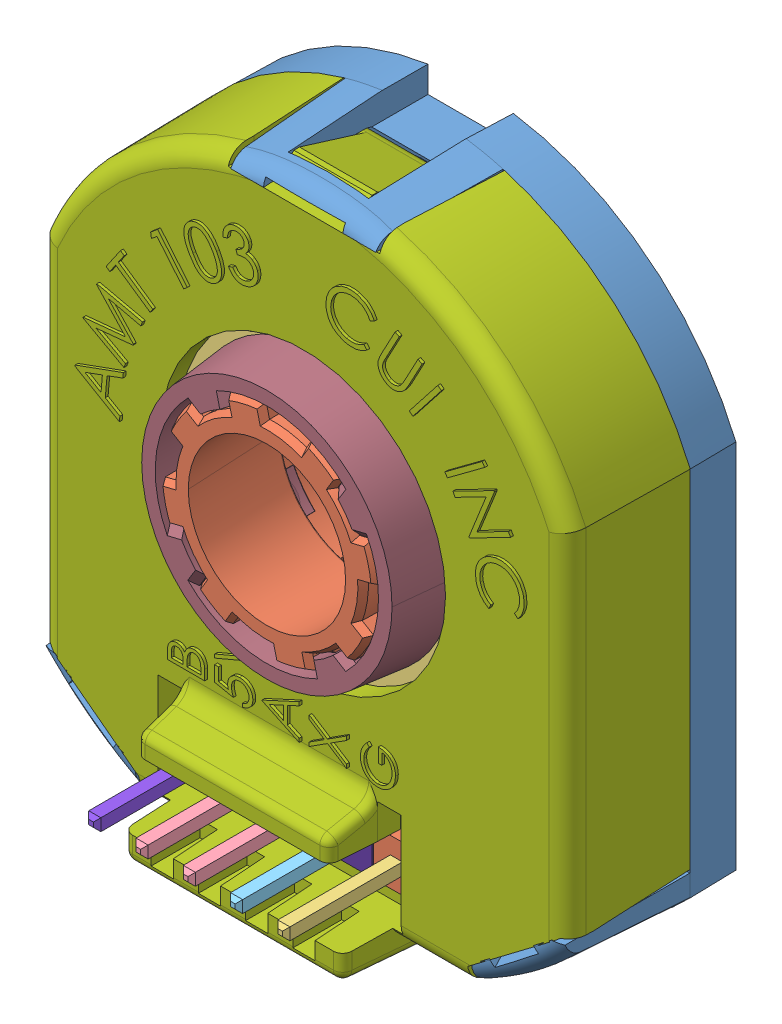
SolidWorks assembly AMT103-V, configuration Default. Lengths in mm.
Overall size (28.68 34.22 14.05).
22 component instances, 22 part files, 5 mates.
Components (placement in the parent):
- AMT103-V3^AMT103-V-1: AMT103-V3^AMT103-V [Default] at (31.6586 0 46.9786) size (28.68 34.14 10.08) (virtual)
- AMT103-V5^AMT103-V-1: AMT103-V5^AMT103-V [Default] at origin size (11.8 12.22 7.8) (virtual)
- AMT103-V7^AMT103-V-1: AMT103-V7^AMT103-V [Default] at origin size (0.65 0.65 6.25) (virtual)
- AMT103-V8^AMT103-V-1: AMT103-V8^AMT103-V [Default] at origin size (0.65 0.65 6.25) (virtual)
- AMT103-V9^AMT103-V-1: AMT103-V9^AMT103-V [Default] at origin size (0.65 0.65 6.25) (virtual)
- AMT103-V10^AMT103-V-1: AMT103-V10^AMT103-V [Default] at origin size (1.67 1.67 2.6) (virtual)
- AMT103-V11^AMT103-V-1: AMT103-V11^AMT103-V [Default] at origin size (28.6 34 9.05) (virtual)
- AMT103-V12^AMT103-V-1: AMT103-V12^AMT103-V [Default] at origin size (0.65 0.65 6.25) (virtual)
- AMT103-V13^AMT103-V-1: AMT103-V13^AMT103-V [Default] at origin size (2.47 2.47 2.5) (virtual)
- AMT103-V14^AMT103-V-1: AMT103-V14^AMT103-V [Default] at origin size (2.47 2.47 2.5) (virtual)
- AMT103-V15^AMT103-V-1: AMT103-V15^AMT103-V [Default] at origin size (1.67 1.67 2.6) (virtual)
- AMT103-V16^AMT103-V-1: AMT103-V16^AMT103-V [Default] at origin size (1.67 1.67 2.6) (virtual)
- AMT103-V17^AMT103-V-1: AMT103-V17^AMT103-V [Default] at origin size (14.07 14.07 6.66) (virtual)
- AMT103-V18^AMT103-V-1: AMT103-V18^AMT103-V [Default] at origin size (1.67 1.67 2.6) (virtual)
- AMT103-V19^AMT103-V-1: AMT103-V19^AMT103-V [Default] at origin size (2.47 2.47 2.5) (virtual)
- AMT103-V21^AMT103-V-1: AMT103-V21^AMT103-V [Default] at origin size (3.37 3.37 1) (virtual)
- AMT103-V22^AMT103-V-1: AMT103-V22^AMT103-V [Default] at origin size (2.47 2.47 2.5) (virtual)
- AMT103-V23^AMT103-V-1: AMT103-V23^AMT103-V [Default] at origin size (26.63 29.52 3.35) (virtual)
- AMT103-V25^AMT103-V-1: AMT103-V25^AMT103-V [Default] at origin size (1.67 1.67 2.6) (virtual)
- AMT103-V27^AMT103-V-1: AMT103-V27^AMT103-V [Default] at origin size (2.47 2.47 2.5) (virtual)
- AMT103-V28^AMT103-V-1: AMT103-V28^AMT103-V [Default] at origin size (25.6 25.6 0.31) (virtual)
- AMT103-V29^AMT103-V-1: AMT103-V29^AMT103-V [Default] at origin size (0.65 0.65 6.25) (virtual)
Mates (geometry in assembly coordinates):
- Concentric1: concentric aligned: cylinder of AMT103-V3^AMT103-V.step-1 through (-0.0526 -0.4184 13.8303) axis (0 0 1) radius 6.3; cone of AMT103-V5^AMT103-V.step-1 through (-0.0526 -0.4184 19.6247) axis (0 0 1)
- Coincident1: coincident anti-aligned: plane of AMT103-V3^AMT103-V.step-1 through (14.2427 -19.2215 16.3303) normal (0 0 1); plane of AMT103-V11^AMT103-V.step-1 through (14.2474 -13.0667 16.3303) normal (0 0 -1)
- Parallel2: parallel aligned: plane of AMT103-V3^AMT103-V.step-1 through (31.6586 0 46.9786) normal (0 1 0)
- Concentric2: concentric aligned: cylinder of AMT103-V4^AMT103-V.step-1 through (-0.0526 -0.4184 19.7531) axis (0 0 1) radius 3.175; cone of AMT103-V5^AMT103-V.step-1 through (-0.0526 -0.4184 19.6247) axis (0 0 1)
- Coincident3: coincident aligned: plane of AMT103-V4^AMT103-V.step-1 through (-3.7738 2.854 24.7799) normal (0 0 1); plane of AMT103-V5^AMT103-V.step-1 through (-4.1894 -7.2968 24.7799) normal (0 0 1)
